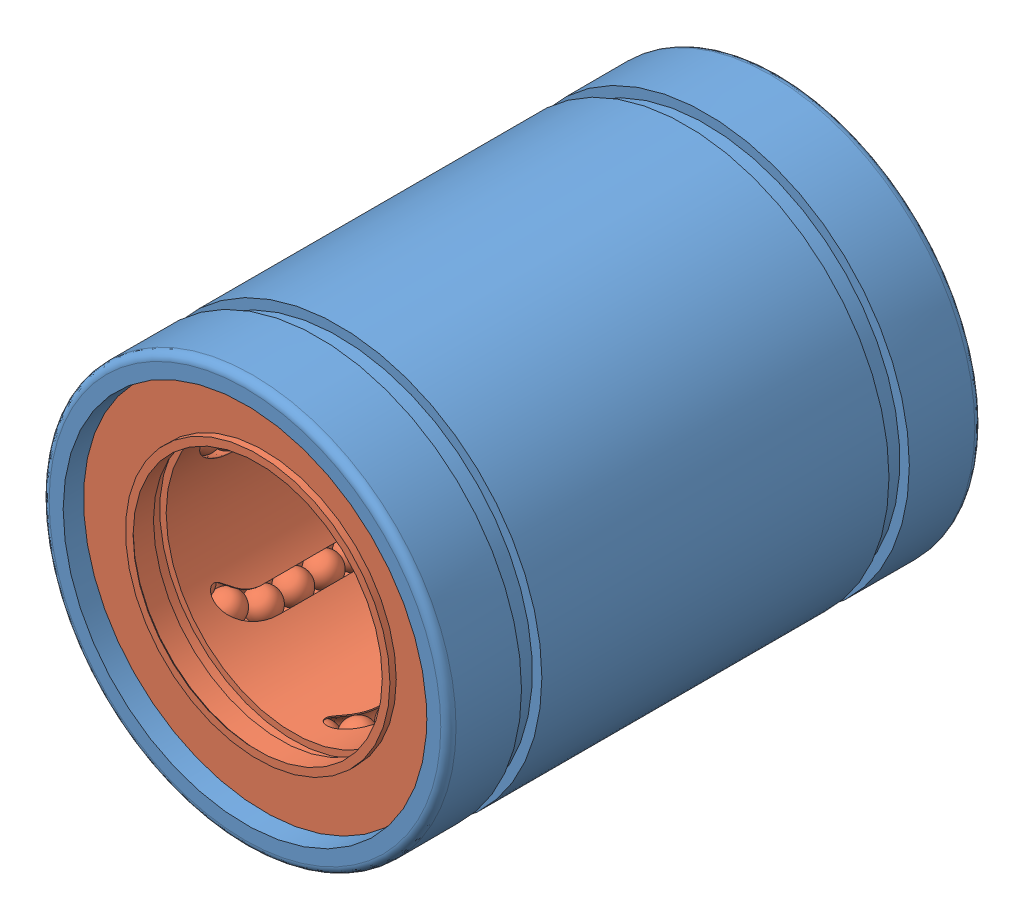
SolidWorks assembly LM20, configuration Default. Lengths in mm.
Overall size (32 32 42).
2 component instances, 2 part files, 2 mates.
Components (placement in the parent):
- LM20-1-1: LM20-1 [Default] at (-2.1463 0.7685 -20.3896) size (32 32 42)
- LM20-2-1: LM20-2 [Default] at (-16.3463 0.7685 20.6104) x (0 0 -1) z (1 0 0) size (40 28.4 28.4)
Mates (geometry in assembly coordinates):
- Concentric1: concentric anti-aligned: cylinder of LM20-1-1 through (-2.1463 0.7685 21.6104) axis (0 0 -1) radius 14.3; cylinder of LM20-2-1 through (-2.1463 0.7685 20.6104) axis (0 0 1) radius 14.2
- Distance1: distance = 1.5 mm aligned: plane of LM20-2-1 through (-16.3463 0.7685 20.1104) normal (0 0 1); plane of LM20-1-1 through (-2.1463 0.7685 21.6104) normal (0 0 1)
